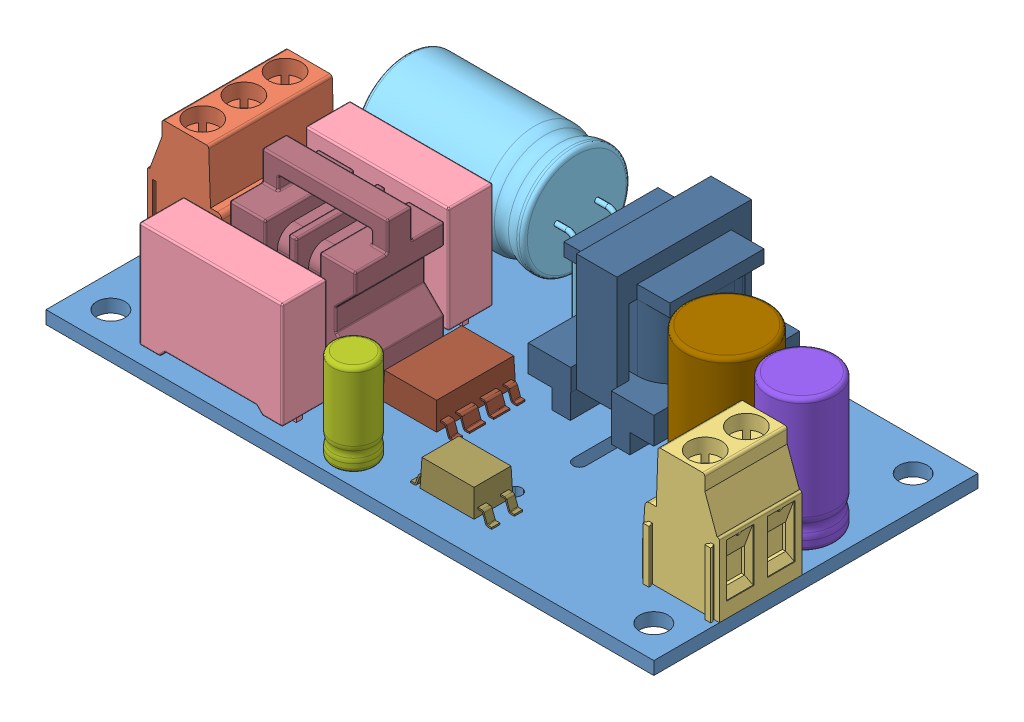
SolidWorks assembly Power Supply Mean Well PS-05-5.virtual, configuration По умолчанию. Lengths in mm.
Overall size (75.31 23.6 40.6).
14 component instances, 13 part files, 39 mates.
Components (placement in the parent):
- Копия text^Power Supply Mean Well PS-05-5.virtual-1: Копия text^Power Supply Mean Well PS-05-5.virtual [По умолчанию] at origin size (75 1.6 40) (virtual)
- Копия 3-pin terminal PC^Power Supply Mean Well PS-05-5.virtual-1: Копия 3-pin terminal PC^Power Supply Mean Well PS-05-5.virtual [Default] at (-35.3941 1.1 -0.12) x (-1 0 0) z (0 0 -1) size (9.64 18.5 15.81) (virtual)
- Копия 2-pin terminal PC^Power Supply Mean Well PS-05-5.virtual-1: Копия 2-pin terminal PC^Power Supply Mean Well PS-05-5.virtual [Default] at (37.5 1.6 11.9) size (9.67 18.5 10.73) (virtual)
- Копия GS-L X2^Power Supply Mean Well PS-05-5.virtual-1: Копия GS-L X2^Power Supply Mean Well PS-05-5.virtual [По умолчанию] at (-27 2.6 13.5) size (17.66 16.6 5.5) (virtual)
- Копия GS-L X2^Power Supply Mean Well PS-05-5.virtual-2: Копия GS-L X2^Power Supply Mean Well PS-05-5.virtual [По умолчанию] at (-27 2.6 -7) size (17.66 16.6 5.5) (virtual)
- Копия conder gs85 22mcf^Power Supply Mean Well PS-05-5.virtual-1: Копия conder gs85 22mcf^Power Supply Mean Well PS-05-5.virtual [По умолчанию] at (-27 10.8 -14) x (0 1 0) z (0 0 -1) size (21.4 23.65 13.2) (virtual)
- Копия conder c30^Power Supply Mean Well PS-05-5.virtual-1: Копия conder c30^Power Supply Mean Well PS-05-5.virtual [По умолчанию] at (-32.5 5.4142 -11.24) size (7.6 9.16 3) (virtual)
- Копия p1416 22mcf^Power Supply Mean Well PS-05-5.virtual-1: Копия p1416 22mcf^Power Supply Mean Well PS-05-5.virtual [По умолчанию] at (-2.34 13.4 17.2) x (-1 0 0) z (0 0 1) size (5.25 14.8 5.25) (virtual)
- Копия gl1404 470mcf^Power Supply Mean Well PS-05-5.virtual-1: Копия gl1404 470mcf^Power Supply Mean Well PS-05-5.virtual [По умолчанию] at (33.15 19 -2.61) x (-1 0 0) z (0 0 1) size (8.25 19.9 8.25) (virtual)
- Копия p1404 1000mcf^Power Supply Mean Well PS-05-5.virtual-1: Копия p1404 1000mcf^Power Supply Mean Well PS-05-5.virtual [По умолчанию] at (23.5 19 -3) x (0 0 -1) z (-1 0 0) size (10.25 19.9 10.25) (virtual)
- Копия trans tf-998zy r1 1415^Power Supply Mean Well PS-05-5.virtual-1: Копия trans tf-998zy r1 1415^Power Supply Mean Well PS-05-5.virtual [По умолчанию] at (2 2.1 0) x (1 0 0) z (0 1 0) size (15.5 18 21.5) (virtual)
- Копия microproc 8p^Power Supply Mean Well PS-05-5.virtual-1: Копия microproc 8p^Power Supply Mean Well PS-05-5.virtual [По умолчанию] at (-6.4552 2.1 9.5) size (9.99 3.8 9.75) (virtual)
- Копия microproc 4p^Power Supply Mean Well PS-05-5.virtual-1: Копия microproc 4p^Power Supply Mean Well PS-05-5.virtual [По умолчанию] at (5.16 2.1 16.5) size (9.99 3.8 4.8) (virtual)
- Копия transformator^Power Supply Mean Well PS-05-5.virtual-1: Копия transformator^Power Supply Mean Well PS-05-5.virtual [По умолчанию] at (-24.84 2.1 10) size (15.5 19.7 11) (virtual)
Mates (geometry in assembly coordinates):
- Coincident1: coincident anti-aligned: plane of Копия text^Power Supply Mean Well PS-05-5.virtual-1 through (0 1.6 0) normal (0 1 0); plane of Копия 3-pin terminal PC^Power Supply Mean Well PS-05-5.virtual-1 through (-32.0108 1.6 -3.8679) normal (0 -1 0)
- Coincident2: coincident aligned: plane of Копия text^Power Supply Mean Well PS-05-5.virtual-1 through (-37.5 1.6 20) normal (-1 0 0); plane of Копия 3-pin terminal PC^Power Supply Mean Well PS-05-5.virtual-1 through (-37.5 3.45 4.88) normal (-1 0 0)
- Distance1: distance = 12.5 mm aligned: plane of Копия 3-pin terminal PC^Power Supply Mean Well PS-05-5.virtual-1 through (5.4564 -18.17 7.5) normal (0 0 1); plane of Копия text^Power Supply Mean Well PS-05-5.virtual-1 through (-37.5 1.6 20) normal (0 0 1)
- Coincident5: coincident anti-aligned: plane of Копия text^Power Supply Mean Well PS-05-5.virtual-1 through (0 1.6 0) normal (0 1 0); plane of Копия 2-pin terminal PC^Power Supply Mean Well PS-05-5.virtual-1 through (32.0108 1.6 8.0279) normal (0 -1 0)
- Coincident6: coincident aligned: plane of Копия text^Power Supply Mean Well PS-05-5.virtual-1 through (37.5 1.6 20) normal (1 0 0); plane of Копия 2-pin terminal PC^Power Supply Mean Well PS-05-5.virtual-1 through (37.5 3.45 4.36) normal (1 0 0)
- Distance2: distance = 8.1 mm aligned: plane of Копия 2-pin terminal PC^Power Supply Mean Well PS-05-5.virtual-1 through (-5.4564 -18.17 11.9) normal (0 0 1); plane of Копия text^Power Supply Mean Well PS-05-5.virtual-1 through (-37.5 1.6 20) normal (0 0 1)
- Distance3: distance = 3.5 mm anti-aligned: plane of Копия transformator^Power Supply Mean Well PS-05-5.virtual-1 through (-24.84 18.2 10) normal (0 0 1); plane of Копия GS-L X2^Power Supply Mean Well PS-05-5.virtual-1 through (-27 2.6 13.5) normal (0 0 -1)
- Distance4: distance = 1 mm aligned: plane of Копия GS-L X2^Power Supply Mean Well PS-05-5.virtual-1 through (-27 2.6 19) normal (0 0 1); plane of Копия text^Power Supply Mean Well PS-05-5.virtual-1 through (-37.5 1.6 20) normal (0 0 1)
- Distance5: distance = 10.5 mm aligned: plane of Копия GS-L X2^Power Supply Mean Well PS-05-5.virtual-1 through (-27 2.6 19) normal (-1 0 0); plane of Копия text^Power Supply Mean Well PS-05-5.virtual-1 through (-37.5 1.6 20) normal (-1 0 0)
- Distance6: distance = 1 mm anti-aligned: plane of Копия GS-L X2^Power Supply Mean Well PS-05-5.virtual-1 through (-27 2.6 19) normal (0 -1 0); plane of Копия text^Power Supply Mean Well PS-05-5.virtual-1 through (0 1.6 0) normal (0 1 0)
- Coincident12: coincident aligned: plane of Копия GS-L X2^Power Supply Mean Well PS-05-5.virtual-1 through (-9.34 2.6 19) normal (1 0 0); plane of Копия transformator^Power Supply Mean Well PS-05-5.virtual-1 through (-9.34 18.2 10) normal (1 0 0)
- Distance7: distance = 0.5 mm anti-aligned: plane of Копия transformator^Power Supply Mean Well PS-05-5.virtual-1 through (-24.84 2.1 10) normal (0 -1 0); plane of Копия text^Power Supply Mean Well PS-05-5.virtual-1 through (0 1.6 0) normal (0 1 0)
- Coincident14: coincident aligned: plane of Копия GS-L X2^Power Supply Mean Well PS-05-5.virtual-1 through (-27 2.6 19) normal (-1 0 0); plane of Копия GS-L X2^Power Supply Mean Well PS-05-5.virtual-2 through (-27 2.6 -1.5) normal (-1 0 0)
- Distance8: distance = 15 mm anti-aligned: plane of Копия GS-L X2^Power Supply Mean Well PS-05-5.virtual-2 through (-27 2.6 -1.5) normal (0 0 1); plane of Копия GS-L X2^Power Supply Mean Well PS-05-5.virtual-1 through (-27 2.6 13.5) normal (0 0 -1)
- Coincident16: coincident aligned: plane of Копия GS-L X2^Power Supply Mean Well PS-05-5.virtual-1 through (-27 15.7 19) normal (0 1 0); plane of Копия GS-L X2^Power Supply Mean Well PS-05-5.virtual-2 through (-27 15.7 -1.5) normal (0 1 0)
- Distance9: distance = 4 mm aligned: plane of Копия conder gs85 22mcf^Power Supply Mean Well PS-05-5.virtual-1 through (-3.65 -4 -16.5) normal (0 -1 0); plane of Копия text^Power Supply Mean Well PS-05-5.virtual-1 through (0 0 0) normal (0 -1 0)
- Distance10: distance = 6 mm aligned: plane of Копия conder gs85 22mcf^Power Supply Mean Well PS-05-5.virtual-1 through (-27 10.8 -14) normal (0 0 -1); plane of Копия text^Power Supply Mean Well PS-05-5.virtual-1 through (-37.5 1.6 -20) normal (0 0 -1)
- Coincident19: coincident aligned: plane of Копия GS-L X2^Power Supply Mean Well PS-05-5.virtual-2 through (-27 2.6 -1.5) normal (-1 0 0); plane of Копия conder gs85 22mcf^Power Supply Mean Well PS-05-5.virtual-1 through (-27 10.8 -14) normal (-1 0 0)
- Distance11: distance = 0.5 mm anti-aligned: plane of Копия p1416 22mcf^Power Supply Mean Well PS-05-5.virtual-1 through (-2.34 2.1 17.2) normal (0 -1 0); plane of Копия text^Power Supply Mean Well PS-05-5.virtual-1 through (0 1.6 0) normal (0 1 0)
- Distance13: distance = 7 mm anti-aligned: plane of Копия p1416 22mcf^Power Supply Mean Well PS-05-5.virtual-1; plane of Копия GS-L X2^Power Supply Mean Well PS-05-5.virtual-1 through (-9.34 2.6 19) normal (1 0 0)
- Distance14: distance = 1.8 mm aligned: plane of Копия p1416 22mcf^Power Supply Mean Well PS-05-5.virtual-1 through (-2.34 13.4 17.2) normal (0 0 1); plane of Копия GS-L X2^Power Supply Mean Well PS-05-5.virtual-1 through (-27 2.6 19) normal (0 0 1)
- Distance15: distance = 0.5 mm anti-aligned: plane of Копия microproc 8p^Power Supply Mean Well PS-05-5.virtual-1 through (-6.4552 2.1 9.5) normal (0 -1 0); plane of Копия text^Power Supply Mean Well PS-05-5.virtual-1 through (0 1.6 0) normal (0 1 0)
- Distance16: distance = 0.5 mm: line of Копия microproc 8p^Power Supply Mean Well PS-05-5.virtual-1 through (-6.4552 2.1 9.5) axis (1 0 0); plane of Копия transformator^Power Supply Mean Well PS-05-5.virtual-1 through (-24.84 18.2 10) normal (0 0 1)
- Distance17: distance = 3 mm: line of Копия microproc 8p^Power Supply Mean Well PS-05-5.virtual-1 through (-6.34 5.4 -0.1348) axis (0 0 1); plane of Копия transformator^Power Supply Mean Well PS-05-5.virtual-1 through (-9.34 18.2 10) normal (1 0 0)
- Coincident28: coincident aligned: plane of Копия microproc 8p^Power Supply Mean Well PS-05-5.virtual-1 through (-6.4552 5.4 9.5) normal (0 1 0); plane of Копия microproc 4p^Power Supply Mean Well PS-05-5.virtual-1 through (5.16 5.4 16.5) normal (0 1 0)
- Distance18: distance = 3.5 mm: line of Копия microproc 4p^Power Supply Mean Well PS-05-5.virtual-1 through (5.16 2.1 16.5) axis (1 0 0); plane of Копия text^Power Supply Mean Well PS-05-5.virtual-1 through (-37.5 1.6 20) normal (0 0 1)
- Distance19: distance = 14.5 mm: line of Копия microproc 4p^Power Supply Mean Well PS-05-5.virtual-1 through (5.16 2.1 11.7) axis (0 0 1); plane of Копия GS-L X2^Power Supply Mean Well PS-05-5.virtual-1 through (-9.34 2.6 19) normal (1 0 0)
- Distance20: distance = 0.5 mm anti-aligned: plane of Копия trans tf-998zy r1 1415^Power Supply Mean Well PS-05-5.virtual-1 through (2 2.1 0) normal (0 -1 0); plane of Копия text^Power Supply Mean Well PS-05-5.virtual-1 through (0 1.6 0) normal (0 1 0)
- Distance21: distance = 20 mm aligned: plane of Копия trans tf-998zy r1 1415^Power Supply Mean Well PS-05-5.virtual-1 through (17.5 19.6 0) normal (1 0 0); plane of Копия text^Power Supply Mean Well PS-05-5.virtual-1 through (37.5 1.6 20) normal (1 0 0)
- Distance22: distance = 2 mm aligned: plane of Копия trans tf-998zy r1 1415^Power Supply Mean Well PS-05-5.virtual-1 through (2 19.6 -18) normal (0 0 -1); plane of Копия text^Power Supply Mean Well PS-05-5.virtual-1 through (-37.5 1.6 -20) normal (0 0 -1)
- Distance23: distance = 1 mm anti-aligned: plane of Копия p1404 1000mcf^Power Supply Mean Well PS-05-5.virtual-1 through (23.5 2.6 -3) normal (0 -1 0); plane of Копия text^Power Supply Mean Well PS-05-5.virtual-1 through (0 1.6 0) normal (0 1 0)
- Distance26: distance = 14 mm anti-aligned: plane of Копия p1404 1000mcf^Power Supply Mean Well PS-05-5.virtual-1 through (23.5 19 -3) normal (-1 0 0); plane of Копия text^Power Supply Mean Well PS-05-5.virtual-1 through (37.5 1.6 20) normal (1 0 0)
- Distance27: distance = 17 mm aligned: plane of Копия p1404 1000mcf^Power Supply Mean Well PS-05-5.virtual-1; plane of Копия text^Power Supply Mean Well PS-05-5.virtual-1 through (-37.5 1.6 -20) normal (0 0 -1)
- Coincident39: coincident aligned: plane of Копия gl1404 470mcf^Power Supply Mean Well PS-05-5.virtual-1 through (33.15 19 -2.61) normal (0 1 0); plane of Копия p1404 1000mcf^Power Supply Mean Well PS-05-5.virtual-1 through (23.5 19 -3) normal (0 1 0)
- Distance28: distance = 4.35 mm anti-aligned: plane of Копия gl1404 470mcf^Power Supply Mean Well PS-05-5.virtual-1; plane of Копия text^Power Supply Mean Well PS-05-5.virtual-1 through (37.5 1.6 20) normal (1 0 0)
- Distance29: distance = 4.35 mm anti-aligned: plane of Копия gl1404 470mcf^Power Supply Mean Well PS-05-5.virtual-1 through (33.15 19 -2.61) normal (0 0 1); plane of Копия 2-pin terminal PC^Power Supply Mean Well PS-05-5.virtual-1 through (-5.4564 -18.17 1.74) normal (0 0 -1)
- Distance30: distance = 1 mm aligned: plane of Копия conder c30^Power Supply Mean Well PS-05-5.virtual-1 through (-36 -1 -11.24) normal (0 -1 0); plane of Копия text^Power Supply Mean Well PS-05-5.virtual-1 through (0 0 0) normal (0 -1 0)
- Distance31: distance = 2 mm anti-aligned: plane of Копия conder c30^Power Supply Mean Well PS-05-5.virtual-1 through (-32.5 5.4142 -9.74) normal (0 0 1); plane of Копия 3-pin terminal PC^Power Supply Mean Well PS-05-5.virtual-1 through (5.4564 -18.17 -7.74) normal (0 0 -1)
- Distance32: distance = 5 mm anti-aligned: plane of Копия conder c30^Power Supply Mean Well PS-05-5.virtual-1 through (-32.5 5.4142 -11.24) normal (1 0 0); plane of Копия text^Power Supply Mean Well PS-05-5.virtual-1 through (-37.5 1.6 20) normal (-1 0 0)
